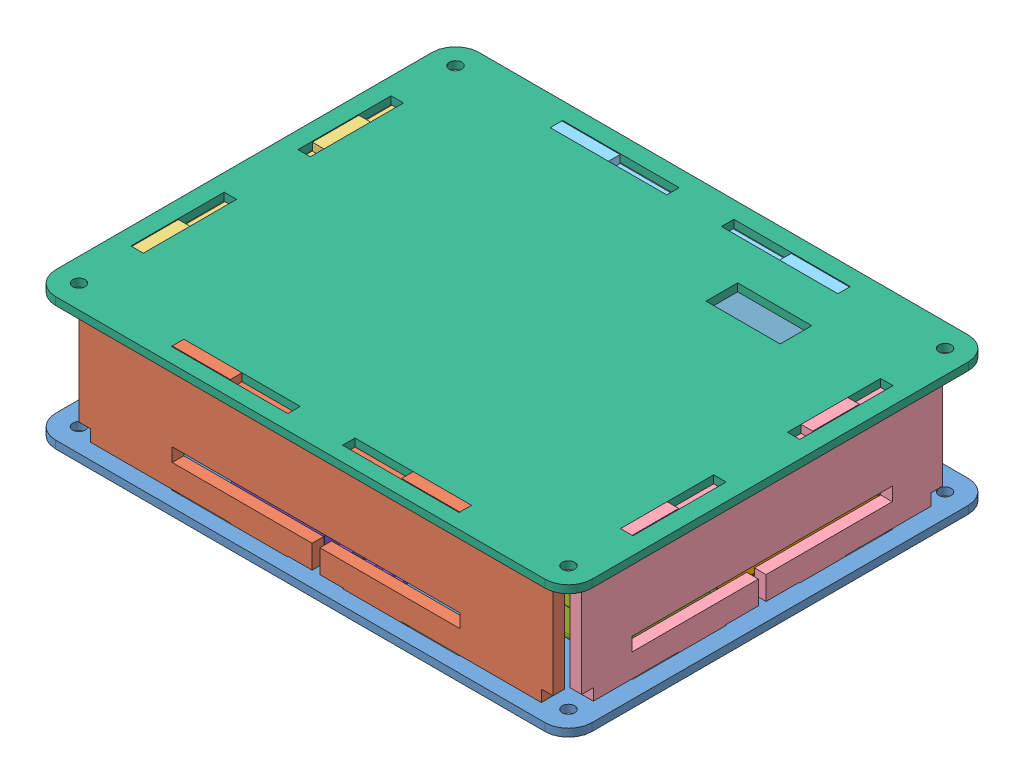
SolidWorks assembly Refreshmate_airfreshner_module_assemble, configuration Default. Lengths in mm.
Overall size (138.1 55.72 109).
221 component instances, 73 part files, 16 mates.
Components (placement in the parent):
- Refreshmate_airfreshner_module_base-2: Refreshmate_airfreshner_module_base [Default] at (-10.0868 60.0989 164.0435) size (138.1 2 109)
- Refreshmate_airfreshner_module_base_connector12 -3: Refreshmate_airfreshner_module_base_connector12  [Default] at (-5.0868 62.0989 157.0294) size (122.1 34 3)
- Refreshmate_airfreshner_module_base_connector_thin_side-2: Refreshmate_airfreshner_module_base_connector_thin_side [Default] at (-5.4868 60.0989 156.0435) size (3 34 93)
- Refreshmate_airfreshner_module_base_connector_thin_side - connector-1: Refreshmate_airfreshner_module_base_connector_thin_side - connector [Default] at (120.4132 60.0989 156.0435) size (3 34 93)
- Refreshmate_airfreshner_module_base_connector1-4: Refreshmate_airfreshner_module_base_connector1 [Default] at (123.0132 62.0989 62.6435) x (-1 0 0) z (0 0 -1) size (122.1 34 3)
- Refreshmate_airfreshner_module_base - upside-1: Refreshmate_airfreshner_module_base - upside [Default] at (-10.0868 92.0989 164.0435) size (138.1 2 109)
- 9V_Battery.step-2: 9V_Battery.step [Default] at (119.9115 70.8489 130.7304) x (0 0 -1) z (0 1 0) size (26.51 49.1 17.51)
- Relay Module-1: Relay Module [Default] at (66.2728 62.0989 164.4867) size (42 14 15)
- Refreshmate_relay_module.step-2: Refreshmate_relay_module.step [Default] at (116.0134 62.5104 67.022) x (-1 0 0) z (0 1 0) size (70.1 49.02 43.82)
  - Board.step-1: Board.step [Default] at origin size (70.1 49.02 0.41)
    - Open CASCADE STEP translator 6.8 2.1.1.step-1: Open CASCADE STEP translator 6.8 2.1.1.step [Default] at (0 0 -0.4115) size (70.1 49.02 0.41)
  - U2.step-1: U2.step [Default] at origin size (4.45 9.97 30.02)
    - 6690172432.step-1: 6690172432.step [Default] at (65.6748 14.3873 0) x (0 -1 0) z (-1 0 0) size (9.97 30.02 4.45)
  - U1.step-1: U1.step [Default] at origin size (4.45 9.97 30.02)
    - 6690172432.step-1: 6690172432.step [Default] at (65.6748 30.4909 0) x (0 -1 0) z (-1 0 0) size (9.97 30.02 4.45)
  - Free-Models.step-1: Free-Models.step [Default] at origin size (67.67 42.76 39.65)
    - ESP-01S_(ESP8266)_Board_Module.step-1: ESP-01S_(ESP8266)_Board_Module.step [Default] at (2.032 8.128 5.08) size (14.8 24.75 11.24)
      - PCB.step-1: PCB.step [Default] at origin size (14.8 24.75 1.2)
      - Antenna.step-1: Antenna.step [Default] at origin size (11.5 6.36 0.02)
      - SerialFlashMem.step-1: SerialFlashMem.step [Default] at origin size (5.2 6.2 1.65)
      - ESP8266EX.step-1: ESP8266EX.step [Default] at origin size (6 6 0.95)
      - Male_Pin_Header_2x4_v5.step-1: Male_Pin_Header_2x4_v5.step [Default] at (3.6324 2.7706 -1.1613) x (1 0 0) z (0 1 0) size (10.21 11.1 5.08)
      - SmalComponent.step-1: SmalComponent.step [Default] at (1.2598 16.5071 0) size (1 0.5 0.5)
      - SmalComponent.step-2: SmalComponent.step [Default] at (3.7598 16.5071 0) size (1 0.5 0.5)
      - SmalComponent.step-3: SmalComponent.step [Default] at (0.9098 14.7571 0) x (0 1 0) z (1 0 0) size (1 0.5 0.5)
      - SmalComponent.step-4: SmalComponent.step [Default] at (1.8098 14.7571 0) x (0 1 0) z (1 0 0) size (1 0.5 0.5)
      - SmalComponent.step-5: SmalComponent.step [Default] at (2.7098 14.7571 0) x (0 1 0) z (1 0 0) size (1 0.5 0.5)
      - SmalComponent.step-6: SmalComponent.step [Default] at (3.6098 14.7571 0) x (0 1 0) z (1 0 0) size (1 0.5 0.5)
      - SmalComponent.step-7: SmalComponent.step [Default] at (4.5098 14.7571 0) x (0 1 0) z (1 0 0) size (1 0.5 0.5)
      - SmalComponent.step-8: SmalComponent.step [Default] at (10.0598 16.6071 0) size (1 0.5 0.5)
      - SmalComponent.step-9: SmalComponent.step [Default] at (12.8598 16.6071 0) size (1 0.5 0.5)
      - SmalComponent.step-10: SmalComponent.step [Default] at (4.7255 6.7248 0) size (1 0.5 0.5)
      - SmalComponent.step-11: SmalComponent.step [Default] at (7.1255 6.7248 0) size (1 0.5 0.5)
      - SmalComponent.step-12: SmalComponent.step [Default] at (1.0098 10.4571 0) x (0 1 0) z (1 0 0) size (1 0.5 0.5)
      - SmalComponent.step-13: SmalComponent.step [Default] at (1.0098 8.2571 0) x (0 1 0) z (1 0 0) size (1 0.5 0.5)
      - SmalComponent.step-14: SmalComponent.step [Default] at (0.9098 12.6571 0) x (0 1 0) z (1 0 0) size (1 0.5 0.5)
      - LargeComponent.step-1: LargeComponent.step [Default] at (1.5052 6.4652 0) size (1.65 0.85 0.85)
      - LED.step-1: LED.step [Default] at (11.974 18.4035 0) size (1.5 0.75 0.75)
      - Crystal.step-1: Crystal.step [Default] at (5.7663 14.7224 0) size (3 2.25 0.75)
    - DO-35.step-1: DO-35.step [Default] at (22.987 22.7832 1.27) x (0 -1 0) z (0 0 1) size (8.12 2.01 5.01)
      - Fillet.step-1: Fillet.step [Default] at origin size (4 2 2)
      - Cylinder001.step-1: Cylinder001.step [Default] at (0.4 0 0) x (0 0 -1) z (1 0 0) size (2.01 2.01 0.8)
      - Cylinder002.step-1: Cylinder002.step [Default] at (2 0 0) x (0 0 -1) z (1 0 0) size (2.01 2.01 0.15)
      - D_DO-35_SOD27_P7.62mm_Horizontal003.step-1: D_DO-35_SOD27_P7.62mm_Horizontal003.step [Default] at (-1.81 0 -1.5) size (8.12 0.5 4.25)
    - LED_RED_3MM.step-1: LED_RED_3MM.step [Default] at (38.3794 41.9608 1.27) x (1 0 0) z (0 -1 0) size (3.9 6.63 3.6)
      - LED_RED_3MM_Pin.step-1: LED_RED_3MM_Pin.step [Default] at (0.0336 -0.3299 0.2064) size (0.8 2.13 3.04)
      - LED_RED_3MM_Body.step-1: LED_RED_3MM_Body.step [Default] at (0.0336 -0.0005 -0.089) size (3.9 5.3 3.6)
    - Resistor_470_Ohm.step-1: Resistor_470_Ohm.step [Default] at (36.068 37.338 1.27) x (1 0 0) z (0 -1 0) size (10.69 26.63 2.45)
    - Capacitor_470uF-16V.step-1: Capacitor_470uF-16V.step [Default] at (58.5724 8.0826 0) x (0 1 0) z (1 0 0) size (8.3 35.4 8.3)
    - Capacitor_100uF-16V.step-1: Capacitor_100uF-16V.step [Default] at (58.5724 15.4686 0) x (0 1 0) z (1 0 0) size (5.3 34.9 5.31)
    - Capacitor_0.1uF-50V.step-1: Capacitor_0.1uF-50V.step [Default] at (58.5724 25.1206 0) x (0 1 0) z (1 0 0) size (4.3 30.9 4.31)
    - Capacitor_0.47uF-50V.step-1: Capacitor_0.47uF-50V.step [Default] at (58.5724 30.5054 0) x (0 1 0) z (1 0 0) size (5.3 34.9 5.31)
    - 1N4005.step-1: 1N4005.step [Default] at (28.3813 20.4998 1.27) x (0 -1 0) z (-1 0 0) size (11.22 5.81 3.01)
    - 1N4005.step-2: 1N4005.step [Default] at (32.7282 20.8309 1.27) x (0 1 0) z (1 0 0) size (11.22 5.81 3.01)
    - 1N4005.step-3: 1N4005.step [Default] at (44.4763 10.4104 1.27) x (1 0 0) z (0 -1 0) size (11.22 5.81 3.01)
    - 1N4005.step-4: 1N4005.step [Default] at (44.1452 6.1976 1.27) x (-1 0 0) z (0 1 0) size (11.22 5.81 3.01)
    - DG301-5.0-02P-12-00AH.step-1: DG301-5.0-02P-12-00AH.step [Default] at (68.1253 36.7067 1.27) x (-1 0 0) z (0 1 0) size (10.6 14.3 7.6)
    - DG301-5.0-02P-12-00AH.step-2: DG301-5.0-02P-12-00AH.step [Default] at (54.23 36.7992 1.27) x (-1 0 0) z (0 1 0) size (10.6 14.3 7.6)
    - RELAY_SRA-05VDC-AL.step-1: RELAY_SRA-05VDC-AL.step [Default] at (44.7294 23.0124 1.27) x (0 -1 0) z (0 0 1) size (16 12.4 17.05)
    - CONNECTOR_BLACK_JST_XH_6_PIN_-_2,54_mm.step-1: CONNECTOR_BLACK_JST_XH_6_PIN_-_2,54_mm.step [Default] at (26.7208 6.6092 1.27) x (0 1 0) z (1 0 0) size (5.73 10 17.96)
    - CONNECTOR_BLACK_JST_XH_4_PIN_-_2,54_mm.step-1: CONNECTOR_BLACK_JST_XH_4_PIN_-_2,54_mm.step [Default] at (3.9018 40.0812 1.27) x (1 0 0) z (0 -1 0) size (5.73 10 12.88)
- PCB_SPS-12-1A_v.03.step-1: PCB_SPS-12-1A_v.03.step [Default] at (14.0091 63.5904 150.0768) x (0 0 -1) z (0 1 0) size (91.5 32.5 26.11)
  - L1.step-1: L1.step [Default] at origin size (3 6.75 14.75)
    - __________________24_Series_-_V.step-1: __________________24_Series_-_V.step [Default] at (13.716 7.239 6) x (0 0 -1) z (1 0 0) size (14.75 6.75 3)
  - R5.step-1: R5.step [Default] at origin size (1.35 2.3 0.75)
    - SMD-R0805.step-1: SMD-R0805.step [Default] at (2.54 -5.8419 -1.4914) x (0 1 0) z (0 0 -1) size (2.3 1.35 0.75)
  - R2.step-1: R2.step [Default] at origin size (1.35 2.3 0.75)
    - SMD-R0805.step-1: SMD-R0805.step [Default] at (18.288 -9.9059 -1.4914) x (0 1 0) z (0 0 -1) size (2.3 1.35 0.75)
  - FU1.step-1: FU1.step [Default] at origin size (7.3 4 18.3)
    - Fuse_D4xL11___KLS5-1011_Series_-_V.step-1: Fuse_D4xL11___KLS5-1011_Series_-_V.step [Default] at (4.358 2.2861 7) x (0 0 -1) z (1 0 0) size (18.3 4 7.3)
      - Fuse_KLS-1011.step-1: Fuse_KLS-1011.step [Default] at origin size (10.3 3.3 3.3)
      - Fuse_KLS-1011-0.step-1: Fuse_KLS-1011-0.step [Default] at (1.15 0 0) size (4.15 3.6 3.6)
      - Fuse_KLS-1011-0.step-2: Fuse_KLS-1011-0.step [Default] at (-1.15 0 0) x (-1 0 0) z (0 0 1) size (4.15 3.6 3.6)
      - Fuse_KLS5-1011.step-1: Fuse_KLS5-1011.step [Default] at (3.5 0 0) size (7 4 4)
      - Fuse_KLS5-1011-1.step-1: Fuse_KLS5-1011-1.step [Default] at (-3.5 0 0) x (-1 0 0) z (0 0 1) size (18.3 4 7.3)
  - XS4.step-1: XS4.step [Default] at origin size (10 10.16 17.3)
    - EK508V-02P.step-1: EK508V-02P.step [Default] at (75.9461 -5.0799 0) x (-1 0 0) z (0 1 0) size (10 17.3 10.16)
  - XS2.step-1: XS2.step [Default] at origin size (10 10.16 17.3)
    - EK508V-02P.step-1: EK508V-02P.step [Default] at (75.9461 15.2401 0) x (-1 0 0) z (0 1 0) size (10 17.3 10.16)
  - XS3.step-1: XS3.step [Default] at origin size (10 10.16 17.3)
    - EK508V-02P.step-1: EK508V-02P.step [Default] at (75.9461 5.0801 0) x (-1 0 0) z (0 1 0) size (10 17.3 10.16)
  - XS1.step-1: XS1.step [Default] at origin size (10 10.16 17.3)
    - EK508V-02P.step-1: EK508V-02P.step [Default] at (10.5409 5.0799 0) x (1 0 0) z (0 -1 0) size (10 17.3 10.16)
  - VU1.step-1: VU1.step [Default] at origin size (7.88 4.59 7)
    - DIP-LTV817_Series.step-1: DIP-LTV817_Series.step [Default] at (42.672 -11.6839 0) x (0 -1 0) z (-1 0 0) size (4.59 7 7.88)
  - VT2.step-1: VT2.step [Default] at origin size (6.69 10.4 2.4)
    - TO-252AA_1.step-1: TO-252AA_1.step [Default] at (27.432 -1.5241 0) x (-1 0 0) z (0 0 1) size (6.69 10.4 2.4)
  - VT1.step-1: VT1.step [Default] at origin size (2.25 2.25 1.11)
    - SOT-363.step-1: SOT-363.step [Default] at (23.3679 -9.9059 -2.2514) x (1 0 0) z (0 0 -1) size (2.25 2.25 1.11)
      - User_Library-TSSOP-6_(SOT-23-6_PITCH_0.65)_pin_TSSOP_tssop6_1.step-1: User_Library-TSSOP-6_(SOT-23-6_PITCH_0.65)_pin_TSSOP_tssop6_1.step [Default] at (0.65 0.675 0) x (-1 0 0) z (0 1 0) size (0.3 0.82 0.45)
      - User_Library-TSSOP-6_(SOT-23-6_PITCH_0.65)_pin_TSSOP_tssop6_1.step-2: User_Library-TSSOP-6_(SOT-23-6_PITCH_0.65)_pin_TSSOP_tssop6_1.step [Default] at (0.65 -0.675 0) x (1 0 0) z (0 -1 0) size (0.3 0.82 0.45)
      - User_Library-TSSOP-6_(SOT-23-6_PITCH_0.65)_pin_TSSOP_tssop6_1.step-3: User_Library-TSSOP-6_(SOT-23-6_PITCH_0.65)_pin_TSSOP_tssop6_1.step [Default] at (-0.65 -0.675 0) x (1 0 0) z (0 -1 0) size (0.3 0.82 0.45)
      - User_Library-TSSOP-6_(SOT-23-6_PITCH_0.65)_pin_TSSOP_tssop6_1.step-4: User_Library-TSSOP-6_(SOT-23-6_PITCH_0.65)_pin_TSSOP_tssop6_1.step [Default] at (0 0.675 0) x (-1 0 0) z (0 1 0) size (0.3 0.82 0.45)
      - User_Library-TSSOP-6_(SOT-23-6_PITCH_0.65)_pin_TSSOP_tssop6_1.step-5: User_Library-TSSOP-6_(SOT-23-6_PITCH_0.65)_pin_TSSOP_tssop6_1.step [Default] at (-0.65 0.675 0) x (-1 0 0) z (0 1 0) size (0.3 0.82 0.45)
      - User_Library-TSSOP-6_(SOT-23-6_PITCH_0.65)_pin_TSSOP_tssop6_1.step-6: User_Library-TSSOP-6_(SOT-23-6_PITCH_0.65)_pin_TSSOP_tssop6_1.step [Default] at (0 -0.675 0) x (1 0 0) z (0 -1 0) size (0.3 0.82 0.45)
      - User_Library-TSSOP-6_(SOT-23-6_PITCH_0.65)_body_TSSOP-6_TSSOP5_1.step-1: User_Library-TSSOP-6_(SOT-23-6_PITCH_0.65)_body_TSSOP-6_TSSOP5_1.step [Default] at origin size (2.25 1.35 1)
  - VD5.step-1: VD5.step [Default] at origin size (5.6 3.95 2.65)
    - DO-214AA.step-1: DO-214AA.step [Default] at (50.392 -11.4301 0) x (1 0 0) z (0 0 1) size (5.6 3.95 2.65)
      - Open CASCADE STEP translator 6.8 1.13.1.1.step-1: Open CASCADE STEP translator 6.8 1.13.1.1.step [Default] at origin size (5.6 3.95 2.65)
      - Open CASCADE STEP translator 6.8 1.13.1.2.step-1: Open CASCADE STEP translator 6.8 1.13.1.2.step [Default] at origin
  - VD4.step-1: VD4.step [Default] at origin size (2.81 5.5 2.6)
    - DO-214AC.step-1: DO-214AC.step [Default] at (35.052 0.0001 -1.4914) x (0 -1 0) z (0 0 -1) size (5.5 2.81 2.6)
  - VD3.step-1: VD3.step [Default] at origin size (2.86 2.3 1.06)
    - SOT-23_1.step-1: SOT-23_1.step [Default] at (41.7221 -0.2201 -1.5514) x (-1 0 0) z (0 -1 0) size (2.86 1.06 2.3)
  - VD2.step-1: VD2.step [Default] at origin size (2.3 2.86 1.06)
    - SOT-23_1.step-1: SOT-23_1.step [Default] at (25.1001 -4.9999 -1.5514) x (0 -1 0) z (1 0 0) size (2.86 1.06 2.3)
  - VD1.step-1: VD1.step [Default] at origin size (7.04 4.95 2.7)
    - DB-1MS_TO-269AA.step-1: DB-1MS_TO-269AA.step [Default] at (6.6041 -3.0481 0) x (1 0 0) z (0 -1 0) size (7.04 2.7 4.95)
  - T1.step-1: T1.step [Default] at origin size (23.02 22.48 20.2)
    - TRANS_-_E20_10_6.step-1: TRANS_-_E20_10_6.step [Default] at (43.8774 -4.7942 6.18) x (1 0 0) z (0 -1 0) size (23.02 20.2 22.48)
      - User_Library-Ensamblaje_FE4528100_2.step-1: User_Library-Ensamblaje_FE4528100_2.step [Default] at (3.8008 6.4163 2.51) x (0 0 -1) z (0 1 0) size (6.63 23.01 7.5)
      - User_Library-Ensamblaje_FE4528100_2.step-2: User_Library-Ensamblaje_FE4528100_2.step [Default] at (-6.2118 6.4163 -17.69) x (0 0 1) z (0 1 0) size (6.63 23.01 7.5)
      - User_Library-Ensamblaje_FE4528070_2.step-1: User_Library-Ensamblaje_FE4528070_2.step [Default] at (-8.8255 -9.7837 0) size (22.04 20.2 21.04)
      - User_Library-Ensamblaje_FE4528056_2.step-1: User_Library-Ensamblaje_FE4528056_2.step [Default] at (8.9945 6.2163 -17.69) x (0 -1 0) z (1 0 0) size (5.9 10.1 20.4)
      - User_Library-Ensamblaje_FE4528056_2.step-2: User_Library-Ensamblaje_FE4528056_2.step [Default] at (8.9945 0.3163 2.51) x (0 1 0) z (1 0 0) size (5.9 10.1 20.4)
      - User_Library-Ensamblaje_Bobinado_2.step-1: User_Library-Ensamblaje_Bobinado_2.step [Default] at (-4.8555 -0.2837 -13.74) size (12 12 12.24)
  - R25.step-1: R25.step [Default] at origin size (1.6 3.1 0.55)
    - SMD_-_R1206_AP214.step-1: SMD_-_R1206_AP214.step [Default] at (77.4701 -9.1199 -1.4914) x (0 1 0) z (-1 0 0) size (3.1 0.55 1.6)
  - R24.step-1: R24.step [Default] at origin size (1.6 3.1 0.55)
    - SMD_-_R1206_AP214.step-1: SMD_-_R1206_AP214.step [Default] at (77.7241 11.2001 -1.4914) x (0 1 0) z (-1 0 0) size (3.1 0.55 1.6)
  - R23.step-1: R23.step [Default] at origin size (1.6 3.1 0.55)
    - SMD_-_R1206_AP214.step-1: SMD_-_R1206_AP214.step [Default] at (3.0479 -12.9301 -1.4914) x (0 -1 0) z (1 0 0) size (3.1 0.55 1.6)
  - R22.step-1: R22.step [Default] at origin size (1.35 2.3 0.75)
    - SMD-R0805.step-1: SMD-R0805.step [Default] at (60.706 -4.826 -1.4914) x (0 1 0) z (0 0 -1) size (2.3 1.35 0.75)
  - R21.step-1: R21.step [Default] at origin size (1.35 2.3 0.75)
    - SMD-R0805.step-1: SMD-R0805.step [Default] at (64.77 -2.794 -1.4914) x (0 1 0) z (0 0 -1) size (2.3 1.35 0.75)
  - R20.step-1: R20.step [Default] at origin size (1.35 2.3 0.75)
    - SMD-R0805.step-1: SMD-R0805.step [Default] at (64.77 1.0161 -1.4914) x (0 1 0) z (0 0 -1) size (2.3 1.35 0.75)
  - R19.step-1: R19.step [Default] at origin size (2.3 1.35 0.75)
    - SMD-R0805.step-1: SMD-R0805.step [Default] at (55.8801 -1.524 -1.4914) x (1 0 0) z (0 0 -1) size (2.3 1.35 0.75)
  - R18.step-1: R18.step [Default] at origin size (1.35 2.3 0.75)
    - SMD-R0805.step-1: SMD-R0805.step [Default] at (49.53 -11.9221 -1.4914) x (0 -1 0) z (0 0 -1) size (2.3 1.35 0.75)
  - R17.step-1: R17.step [Default] at origin size (2.3 1.35 0.75)
    - SMD-R0805.step-1: SMD-R0805.step [Default] at (52.832 -12.954 -1.4914) x (1 0 0) z (0 0 -1) size (2.3 1.35 0.75)
  - R16.step-1: R16.step [Default] at origin size (2.3 1.35 0.75)
    - SMD-R0805.step-1: SMD-R0805.step [Default] at (52.832 -9.906 -1.4914) x (1 0 0) z (0 0 -1) size (2.3 1.35 0.75)
  - R15.step-1: R15.step [Default] at origin size (1.6 3.1 0.55)
    - SMD_-_R1206_AP214.step-1: SMD_-_R1206_AP214.step [Default] at (25.1459 4.8019 -1.4914) x (0 -1 0) z (1 0 0) size (3.1 0.55 1.6)
  - R14.step-1: R14.step [Default] at origin size (1.35 2.3 0.75)
    - SMD-R0805.step-1: SMD-R0805.step [Default] at (18.288 -5.8419 -1.4914) x (0 1 0) z (0 0 -1) size (2.3 1.35 0.75)
  - R13.step-1: R13.step [Default] at origin size (2.3 1.35 0.75)
    - SMD-R0805.step-1: SMD-R0805.step [Default] at (25.1461 -1.524 -1.4914) x (1 0 0) z (0 0 -1) size (2.3 1.35 0.75)
  - R12.step-1: R12.step [Default] at origin size (3.3 6.4 0.65)
    - SMD-R2512.step-1: SMD-R2512.step [Default] at (30.9881 7.3661 -1.4914) x (0 1 0) z (0 0 -1) size (6.4 3.3 0.65)
      - Open CASCADE STEP translator 6.8 1.32.1.1.step-1: Open CASCADE STEP translator 6.8 1.32.1.1.step [Default] at origin size (6.4 3.3 0.65)
      - Open CASCADE STEP translator 6.8 1.32.1.2.step-1: Open CASCADE STEP translator 6.8 1.32.1.2.step [Default] at origin
  - R11.step-1: R11.step [Default] at origin size (2.3 1.35 0.75)
    - SMD-R0805.step-1: SMD-R0805.step [Default] at (25.1461 0.762 -1.4914) x (1 0 0) z (0 0 -1) size (2.3 1.35 0.75)
  - R10.step-1: R10.step [Default] at origin size (1.6 3.1 0.55)
    - SMD_-_R1206_AP214.step-1: SMD_-_R1206_AP214.step [Default] at (41.6559 4.5479 -1.4914) x (0 -1 0) z (1 0 0) size (3.1 0.55 1.6)
  - R9.step-1: R9.step [Default] at origin size (1.35 2.3 0.75)
    - SMD-R0805.step-1: SMD-R0805.step [Default] at (31.242 -11.4139 -1.4914) x (0 1 0) z (0 0 -1) size (2.3 1.35 0.75)
  - R8.step-1: R8.step [Default] at origin size (1.35 2.3 0.75)
    - SMD-R0805.step-1: SMD-R0805.step [Default] at (33.782 -11.43 -1.4914) x (0 1 0) z (0 0 -1) size (2.3 1.35 0.75)
  - R7.step-1: R7.step [Default] at origin size (2.3 1.35 0.75)
    - SMD-R0805.step-1: SMD-R0805.step [Default] at (23.8761 -13.716 -1.4914) x (1 0 0) z (0 0 -1) size (2.3 1.35 0.75)
  - R6.step-1: R6.step [Default] at origin size (3.3 6.4 0.65)
    - SMD-R2512.step-1: SMD-R2512.step [Default] at (18.5421 10.7951 -1.4914) x (0 1 0) z (0 0 -1) size (6.4 3.3 0.65)
      - Open CASCADE STEP translator 6.8 1.32.1.1.step-1: Open CASCADE STEP translator 6.8 1.32.1.1.step [Default] at origin size (6.4 3.3 0.65)
      - Open CASCADE STEP translator 6.8 1.32.1.2.step-1: Open CASCADE STEP translator 6.8 1.32.1.2.step [Default] at origin
  - R4.step-1: R4.step [Default] at origin size (1.35 2.3 0.75)
    - SMD-R0805.step-1: SMD-R0805.step [Default] at (20.828 -5.8419 -1.4914) x (0 1 0) z (0 0 -1) size (2.3 1.35 0.75)
  - R3.step-1: R3.step [Default] at origin size (1.35 2.3 0.75)
    - SMD-R0805.step-1: SMD-R0805.step [Default] at (25.908 -9.9059 -1.4914) x (0 1 0) z (0 0 -1) size (2.3 1.35 0.75)
  - R1.step-1: R1.step [Default] at origin size (1.35 2.3 0.75)
    - SMD-R0805.step-1: SMD-R0805.step [Default] at (20.828 -9.9059 -1.4914) x (0 1 0) z (0 0 -1) size (2.3 1.35 0.75)
  - L3.step-1: L3.step [Default] at origin size (4.58 10.39 14)
    - Inductors_EMI_9x5x3.step-1: Inductors_EMI_9x5x3.step [Default] at (71.8819 1.2701 0.03) x (0 -1 0) z (0 0 1) size (10.39 4.58 14)
  - L2.step-1: L2.step [Default] at origin size (8.7 8.7 14.99)
    - Induct___RLB-0914.step-1: Induct___RLB-0914.step [Default] at (59.7301 2.0321 0) x (1 0 0) z (0 -1 0) size (8.7 14.99 8.7)
  - HL1.step-1: HL1.step [Default] at origin size (6 5.5 15.44)
    - LED-D5G.step-1: LED-D5G.step [Default] at (5.7151 -12.7 4) x (0 1 0) z (1 0 0) size (5.5 15.44 6)
  - DD1.step-1: DD1.step [Default] at origin size (5 6.2 1.75)
    - SOIC-8______MS-012AA.step-1: SOIC-8______MS-012AA.step [Default] at (13.462 -7.6199 -1.4914) x (-1 0 0) z (0 0 -1) size (5 6.2 1.75)
      - Open CASCADE STEP translator 6.8 1.45.1.1.step-1: Open CASCADE STEP translator 6.8 1.45.1.1.step [Default] at origin size (5 6.2 1.75)
      - Open CASCADE STEP translator 6.8 1.45.1.2.step-1: Open CASCADE STEP translator 6.8 1.45.1.2.step [Default] at origin
  - DA1.step-1: DA1.step [Default] at origin size (3 3 1.46)
    - SOT-23-5_____0,95.step-1: SOT-23-5_____0,95.step [Default] at (56.8961 -4.8259 -2.4514) x (0 -1 0) z (0 0 -1) size (3 3 1.46)
      - User_Library-SOT-23-5_pin_SOT_sot-23-6_1.step-1: User_Library-SOT-23-5_pin_SOT_sot-23-6_1.step [Default] at (0 0.875 0) x (-1 0 0) z (0 1 0) size (0.4 1.02 0.62)
      - User_Library-SOT-23-5_pin_SOT_sot-23-6_1.step-2: User_Library-SOT-23-5_pin_SOT_sot-23-6_1.step [Default] at (-0.95 -0.875 0) x (1 0 0) z (0 -1 0) size (0.4 1.02 0.62)
      - User_Library-SOT-23-5_body_sot23-6_1.step-1: User_Library-SOT-23-5_body_sot23-6_1.step [Default] at origin size (3 1.75 1.3)
      - User_Library-SOT-23-5_pin_SOT_sot-23-6_1.step-3: User_Library-SOT-23-5_pin_SOT_sot-23-6_1.step [Default] at (0.95 -0.875 0) x (1 0 0) z (0 -1 0) size (0.4 1.02 0.62)
      - User_Library-SOT-23-5_pin_SOT_sot-23-6_1.step-4: User_Library-SOT-23-5_pin_SOT_sot-23-6_1.step [Default] at (-0.95 0.875 0) x (-1 0 0) z (0 1 0) size (0.4 1.02 0.62)
      - User_Library-SOT-23-5_pin_SOT_sot-23-6_1.step-5: User_Library-SOT-23-5_pin_SOT_sot-23-6_1.step [Default] at (0.95 0.875 0) x (-1 0 0) z (0 1 0) size (0.4 1.02 0.62)
  - C18.step-1: C18.step [Default] at origin size (1.2 2 1.2)
    - SMD-C0805.step-1: SMD-C0805.step [Default] at (77.9781 0.0001 -1.4914) x (0 1 0) z (0 0 -1) size (2 1.2 1.2)
  - C17.step-1: C17.step [Default] at origin size (1.2 2 1.2)
    - SMD-C0805.step-1: SMD-C0805.step [Default] at (73.4059 1.2699 -1.4914) x (0 -1 0) z (0 0 -1) size (2 1.2 1.2)
  - C16.step-1: C16.step [Default] at origin size (1.2 2 1.2)
    - SMD-C0805.step-1: SMD-C0805.step [Default] at (70.3579 1.2699 -1.4914) x (0 -1 0) z (0 0 -1) size (2 1.2 1.2)
  - C15.step-1: C15.step [Default] at origin size (10.5 10.5 20.02)
    - Cap_-_EL(10x16-5).step-1: Cap_-_EL(10x16-5).step [Default] at (65.2781 10.16 0) size (10.5 10.5 20.02)
  - C14.step-1: C14.step [Default] at origin size (2 1.2 1.2)
    - SMD-C0805.step-1: SMD-C0805.step [Default] at (59.6901 -1.5241 -1.4914) x (1 0 0) z (0 0 -1) size (2 1.2 1.2)
  - C13.step-1: C13.step [Default] at origin size (13 13 24.51)
    - Cap_-_EL(12.5x20-5).step-1: Cap_-_EL(12.5x20-5).step [Default] at (64.0481 -8.636 0) x (1 0 0) z (0 0 1) size (13 13 24.51)
  - C12.step-1: C12.step [Default] at origin size (1.2 2 1.2)
    - SMD-C0805.step-1: SMD-C0805.step [Default] at (56.1339 -11.9381 -1.4914) x (0 -1 0) z (0 0 -1) size (2 1.2 1.2)
  - C11.step-1: C11.step [Default] at origin size (3.2 1.6 0.78)
    - SMD-C1206.step-1: SMD-C1206.step [Default] at (46.4821 6.8579 -1.8814) x (1 0 0) z (0 1 0) size (3.2 0.78 1.6)
  - C10.step-1: C10.step [Default] at origin size (2.5 3.2 0.78)
    - SMD-C1210.step-1: SMD-C1210.step [Default] at (35.0521 5.842 -1.8814) x (0 1 0) z (-1 0 0) size (3.2 0.78 2.5)
  - C9.step-1: C9.step [Default] at origin size (1.2 2 1.2)
    - SMD-C0805.step-1: SMD-C0805.step [Default] at (9.3979 -9.9061 -1.4914) x (0 -1 0) z (0 0 -1) size (2 1.2 1.2)
  - C8.step-1: C8.step [Default] at origin size (8.21 8 15.6)
    - Cap_-_EL(8x12-3_5)T.step-1: Cap_-_EL(8x12-3_5)T.step [Default] at (16.0021 -0.2541 0) x (0 -1 0) z (0 0 1) size (8.21 8 15.6)
  - C7.step-1: C7.step [Default] at origin size (1.2 2 1.2)
    - SMD-C0805.step-1: SMD-C0805.step [Default] at (18.5421 0.5081 -1.4914) x (0 1 0) z (0 0 -1) size (2 1.2 1.2)
  - C6.step-1: C6.step [Default] at origin size (1.2 2 1.2)
    - SMD-C0805.step-1: SMD-C0805.step [Default] at (9.3979 -5.8421 -1.4914) x (0 -1 0) z (0 0 -1) size (2 1.2 1.2)
  - C5.step-1: C5.step [Default] at origin size (1.2 2 1.2)
    - SMD-C0805.step-1: SMD-C0805.step [Default] at (4.8259 -5.8421 -1.4914) x (0 -1 0) z (0 0 -1) size (2 1.2 1.2)
  - C4.step-1: C4.step [Default] at origin size (1.2 2 1.2)
    - SMD-C0805.step-1: SMD-C0805.step [Default] at (28.1941 -9.9059 -1.4914) x (0 1 0) z (0 0 -1) size (2 1.2 1.2)
  - C3.step-1: C3.step [Default] at origin size (1.2 2 1.2)
    - SMD-C0805.step-1: SMD-C0805.step [Default] at (7.1119 -5.8421 -1.4914) x (0 -1 0) z (0 0 -1) size (2 1.2 1.2)
  - C2.step-1: C2.step [Default] at origin size (2 1.2 1.2)
    - SMD-C0805.step-1: SMD-C0805.step [Default] at (19.3041 -12.9541 -1.4914) x (1 0 0) z (0 0 -1) size (2 1.2 1.2)
  - C1.step-1: C1.step [Default] at origin size (10.2 10 23.31)
    - Cap_-_EL(10x20-5).step-1: Cap_-_EL(10x20-5).step [Default] at (22.3519 9.272 0) x (0 -1 0) z (0 0 1) size (10.2 10 23.31)
  - Board.step-1: Board.step [Default] at origin size (86.5 32.5 1.49)
Mates (geometry in assembly coordinates):
- Coincident14: coincident anti-aligned: plane of Refreshmate_airfreshner_module_base-2 through (66.0132 62.0989 157.0294) normal (1 0 0); plane of Refreshmate_airfreshner_module_base_connector12 -3 through (66.0132 62.0989 160.0294) normal (-1 0 0)
- Coincident15: coincident anti-aligned: line of Refreshmate_airfreshner_module_base-2 through (96.0132 60.0989 157.0294) axis (-1 0 0); line of Refreshmate_airfreshner_module_base_connector12 -3 through (66.0132 60.0989 157.0294) axis (1 0 0)
- Coincident16: coincident anti-aligned: plane of Refreshmate_airfreshner_module_base-2 through (-5.6868 62.0989 100.0435) normal (0 0 -1); plane of Refreshmate_airfreshner_module_base_connector_thin_side-2 through (-2.4868 60.0989 100.0435) normal (0 0 1)
- Coincident17: coincident aligned: line of Refreshmate_airfreshner_module_base-2 through (-2.4868 60.0989 100.0435) axis (0 0 -1); line of Refreshmate_airfreshner_module_base_connector_thin_side-2 through (-2.4868 60.0989 100.0435) axis (0 0 -1)
- Coincident18: coincident anti-aligned: plane of Refreshmate_airfreshner_module_base-2 through (120.4132 62.0989 100.0435) normal (0 0 -1); plane of Refreshmate_airfreshner_module_base_connector_thin_side - connector-1 through (123.4132 60.0989 100.0435) normal (0 0 1)
- Coincident19: coincident anti-aligned: line of Refreshmate_airfreshner_module_base-2 through (120.4132 60.0989 76.0435) axis (0 0 1); line of Refreshmate_airfreshner_module_base_connector_thin_side - connector-1 through (120.4132 60.0989 100.0435) axis (0 0 -1)
- Coincident25: coincident anti-aligned: plane of Refreshmate_airfreshner_module_base-2 through (66.0132 62.0989 59.4435) normal (1 0 0); plane of Refreshmate_airfreshner_module_base_connector1-4 through (66.0132 62.0989 59.6435) normal (-1 0 0)
- Coincident26: coincident anti-aligned: line of Refreshmate_airfreshner_module_base-2 through (66.0132 60.0989 62.6435) axis (1 0 0); line of Refreshmate_airfreshner_module_base_connector1-4 through (81.0132 60.0989 62.6435) axis (-1 0 0)
- Coincident27: coincident aligned: plane of Refreshmate_airfreshner_module_base-2 through (-10.0868 60.0989 164.0435) normal (0 -1 0); plane of Refreshmate_airfreshner_module_base_connector1-4 through (123.0132 60.0989 59.6435) normal (0 -1 0)
- Concentric2: concentric aligned: cylinder of Refreshmate_airfreshner_module_base-2 through (-4.0868 62.0989 61.0435) axis (0 -1 0) radius 1.6; cylinder of Refreshmate_airfreshner_module_base - upside-1 through (-4.0868 94.0989 61.0435) axis (0 -1 0) radius 1.6
- Coincident28: coincident aligned: plane of Refreshmate_airfreshner_module_base_connector12 -3 through (-5.0868 94.0989 160.0294) normal (0 1 0); plane of Refreshmate_airfreshner_module_base - upside-1 through (-10.0868 94.0989 164.0435) normal (0 1 0)
- Coincident35: coincident anti-aligned: plane of Refreshmate_airfreshner_module_base-2 through (-10.0868 62.0989 164.0435) normal (0 1 0); plane of Relay Module-1 through (39.1067 62.0989 159.2552) normal (0 -1 0)
- Coincident36: coincident anti-aligned: cylinder of Refreshmate_airfreshner_module_base-2 through (122.0132 62.0989 158.0435) axis (0 -1 0) radius 1.6; circle of Refreshmate_airfreshner_module_base - upside-1
- Coincident37: coincident anti-aligned: plane of Refreshmate_airfreshner_module_base-2 through (-10.0868 62.0989 164.0435) normal (0 1 0); plane of Refreshmate_relay_module.step-2/Board.step-1/Open CASCADE STEP translator 6.8 2.1.1.step-1 through (116.0134 62.0989 67.022) normal (0 -1 0)
- Concentric3: concentric aligned: circle of Refreshmate_airfreshner_module_base-2; circle of Refreshmate_relay_module.step-2/Board.step-1/Open CASCADE STEP translator 6.8 2.1.1.step-1
- Coincident38: coincident anti-aligned: plane of Refreshmate_airfreshner_module_base-2 through (-10.0868 62.0989 164.0435) normal (0 1 0); plane of PCB_SPS-12-1A_v.03.step-1/Board.step-1 through (30.2921 62.0989 150.0818) normal (0 -1 0)
